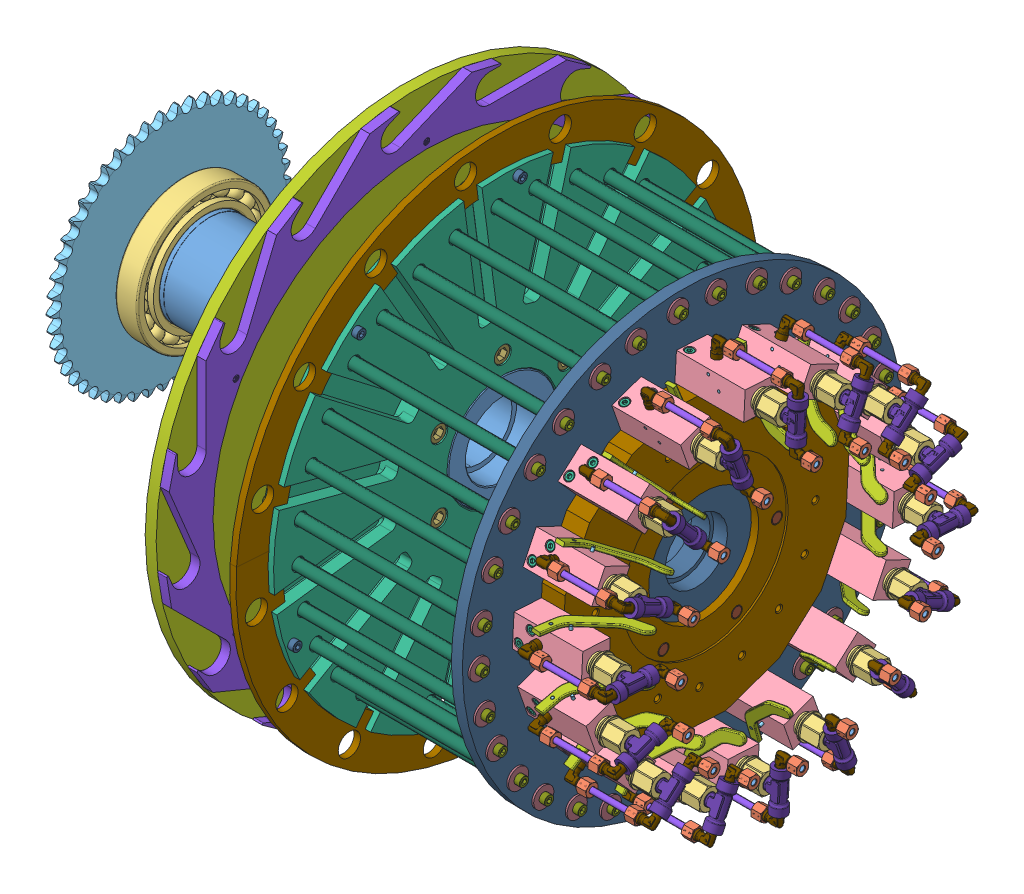
SolidWorks assembly assieme parte rotante, configuration Default. Lengths in mm. (continued)
Components (placement in the parent): (continued)
- AssiemeValvola-7: AssiemeValvola [Default] at (515.3257 -134.8578 488.6421) x (0 0.901303 -0.433189) z (0 -0.433189 -0.901303) size (90.26 138.63 38)
  - RaccordoT-1: RaccordoT [Default] at origin size (43 29.75 16.5)
  - Raccordo a L-1: Raccordo a L [Default] at (-30 0 0) x (0 -1 0) z (0 0 -1) size (28.34 25.51 14.01)
    - 1809_06_10_01-1: 1809_06_10_01 [Default] at origin size (22.49 23 10)
    - 1809_06_10_02-1: 1809_06_10_02 [Default] at origin size (6.5 8.5 8.5)
    - 1809_06_10_03-1: 1809_06_10_03 [Default] at origin size (11.02 15.01 14.01)
  - Raccordo a L-2: Raccordo a L [Default] at (30 0 0) x (0 1 0) z (0 0 -1) size (28.34 25.51 14.01)
    - 1809_06_10_01-1: 1809_06_10_01 [Default] at origin size (22.49 23 10)
    - 1809_06_10_02-1: 1809_06_10_02 [Default] at origin size (6.5 8.5 8.5)
    - 1809_06_10_03-1: 1809_06_10_03 [Default] at origin size (11.02 15.01 14.01)
  - TappoChiusura-1: TappoChiusura [Default] at (0 -32 0) x (0 -1 0) z (0 0 1) size (38.28 26.74 26.74)
  - CorpoValvola-1: CorpoValvola [Default] at (-15 -115.2824 0) size (30 75 34)
  - Raccordo a L-3: Raccordo a L [Default] at (-30 -88.2824 0) x (0 1 0) z (0 0 1) size (28.34 25.51 14.01)
    - 1809_06_10_01-1: 1809_06_10_01 [Default] at origin size (22.49 23 10)
    - 1809_06_10_02-1: 1809_06_10_02 [Default] at origin size (6.5 8.5 8.5)
    - 1809_06_10_03-1: 1809_06_10_03 [Default] at origin size (11.02 15.01 14.01)
  - Spina_3x38-1: Spina_3x38 [Default] at (0 -68.2824 -21) x (-1 0 0) z (0 0 1) size (3 3 38)
  - Spina_3x38-2: Spina_3x38 [Default] at (-10 -80.2824 -21) x (0.996193 0.087174 0) z (0 0 1) size (3 3 38)
  - M5 40mm-3: M5 40mm [ISO 4762 M5 x 40 - 40N] at (-14.6 -108.7824 9) size (45 8.5 8.5)
  - M5 40mm-2: M5 40mm [ISO 4762 M5 x 40 - 40N] at (-14.6 -96.7824 -9) size (45 8.5 8.5)
  - LevaValvola-1: LevaValvola [Default] at (-24.507 -86.571 -17) x (0.996193 0.087174 0) z (0 0 1) size (77.55 60.2 4)
  - Tubo-1: Tubo [Default] at (-30 -15.9665 0) x (1 0 0) z (0 -1 0) size (6 6 56.4)
- AssiemeValvola-8: AssiemeValvola [Default] at (515.3257 -95.0129 541.6718) x (0 0.666921 -0.745128) z (0 -0.745128 -0.666921) size (90.26 138.63 38)
  - RaccordoT-1: RaccordoT [Default] at origin size (43 29.75 16.5)
  - Raccordo a L-1: Raccordo a L [Default] at (-30 0 0) x (0 -1 0) z (0 0 -1) size (28.34 25.51 14.01)
    - 1809_06_10_01-1: 1809_06_10_01 [Default] at origin size (22.49 23 10)
    - 1809_06_10_02-1: 1809_06_10_02 [Default] at origin size (6.5 8.5 8.5)
    - 1809_06_10_03-1: 1809_06_10_03 [Default] at origin size (11.02 15.01 14.01)
  - Raccordo a L-2: Raccordo a L [Default] at (30 0 0) x (0 1 0) z (0 0 -1) size (28.34 25.51 14.01)
    - 1809_06_10_01-1: 1809_06_10_01 [Default] at origin size (22.49 23 10)
    - 1809_06_10_02-1: 1809_06_10_02 [Default] at origin size (6.5 8.5 8.5)
    - 1809_06_10_03-1: 1809_06_10_03 [Default] at origin size (11.02 15.01 14.01)
  - TappoChiusura-1: TappoChiusura [Default] at (0 -32 0) x (0 -1 0) z (0 0 1) size (38.28 26.74 26.74)
  - CorpoValvola-1: CorpoValvola [Default] at (-15 -115.2824 0) size (30 75 34)
  - Raccordo a L-3: Raccordo a L [Default] at (-30 -88.2824 0) x (0 1 0) z (0 0 1) size (28.34 25.51 14.01)
    - 1809_06_10_01-1: 1809_06_10_01 [Default] at origin size (22.49 23 10)
    - 1809_06_10_02-1: 1809_06_10_02 [Default] at origin size (6.5 8.5 8.5)
    - 1809_06_10_03-1: 1809_06_10_03 [Default] at origin size (11.02 15.01 14.01)
  - Spina_3x38-1: Spina_3x38 [Default] at (0 -68.2824 -21) x (-1 0 0) z (0 0 1) size (3 3 38)
  - Spina_3x38-2: Spina_3x38 [Default] at (-10 -80.2824 -21) x (0.996193 0.087174 0) z (0 0 1) size (3 3 38)
  - M5 40mm-3: M5 40mm [ISO 4762 M5 x 40 - 40N] at (-14.6 -108.7824 9) size (45 8.5 8.5)
  - M5 40mm-2: M5 40mm [ISO 4762 M5 x 40 - 40N] at (-14.6 -96.7824 -9) size (45 8.5 8.5)
  - LevaValvola-1: LevaValvola [Default] at (-24.507 -86.571 -17) x (0.996193 0.087174 0) z (0 0 1) size (77.55 60.2 4)
  - Tubo-1: Tubo [Default] at (-30 -15.9665 0) x (1 0 0) z (0 -1 0) size (6 6 56.4)
- AssiemeValvola-9: AssiemeValvola [Default] at (515.3257 -37.9074 575.4168) x (0 0.331007 -0.943628) z (0 -0.943628 -0.331007) size (90.26 138.63 38)
  - RaccordoT-1: RaccordoT [Default] at origin size (43 29.75 16.5)
  - Raccordo a L-1: Raccordo a L [Default] at (-30 0 0) x (0 -1 0) z (0 0 -1) size (28.34 25.51 14.01)
    - 1809_06_10_01-1: 1809_06_10_01 [Default] at origin size (22.49 23 10)
    - 1809_06_10_02-1: 1809_06_10_02 [Default] at origin size (6.5 8.5 8.5)
    - 1809_06_10_03-1: 1809_06_10_03 [Default] at origin size (11.02 15.01 14.01)
  - Raccordo a L-2: Raccordo a L [Default] at (30 0 0) x (0 1 0) z (0 0 -1) size (28.34 25.51 14.01)
    - 1809_06_10_01-1: 1809_06_10_01 [Default] at origin size (22.49 23 10)
    - 1809_06_10_02-1: 1809_06_10_02 [Default] at origin size (6.5 8.5 8.5)
    - 1809_06_10_03-1: 1809_06_10_03 [Default] at origin size (11.02 15.01 14.01)
  - TappoChiusura-1: TappoChiusura [Default] at (0 -32 0) x (0 -1 0) z (0 0 1) size (38.28 26.74 26.74)
  - CorpoValvola-1: CorpoValvola [Default] at (-15 -115.2824 0) size (30 75 34)
  - Raccordo a L-3: Raccordo a L [Default] at (-30 -88.2824 0) x (0 1 0) z (0 0 1) size (28.34 25.51 14.01)
    - 1809_06_10_01-1: 1809_06_10_01 [Default] at origin size (22.49 23 10)
    - 1809_06_10_02-1: 1809_06_10_02 [Default] at origin size (6.5 8.5 8.5)
    - 1809_06_10_03-1: 1809_06_10_03 [Default] at origin size (11.02 15.01 14.01)
  - Spina_3x38-1: Spina_3x38 [Default] at (0 -68.2824 -21) x (-1 0 0) z (0 0 1) size (3 3 38)
  - Spina_3x38-2: Spina_3x38 [Default] at (-10 -80.2824 -21) x (0.996193 0.087174 0) z (0 0 1) size (3 3 38)
  - M5 40mm-3: M5 40mm [ISO 4762 M5 x 40 - 40N] at (-14.6 -108.7824 9) size (45 8.5 8.5)
  - M5 40mm-2: M5 40mm [ISO 4762 M5 x 40 - 40N] at (-14.6 -96.7824 -9) size (45 8.5 8.5)
  - LevaValvola-1: LevaValvola [Default] at (-24.507 -86.571 -17) x (0.996193 0.087174 0) z (0 0 1) size (77.55 60.2 4)
  - Tubo-1: Tubo [Default] at (-30 -15.9665 0) x (1 0 0) z (0 -1 0) size (6 6 56.4)
- AssiemeValvola-10: AssiemeValvola [Default] at (515.3257 27.7648 584.7399) x (0 -0.055301 -0.99847) z (0 -0.99847 0.055301) size (90.26 138.63 38)
  - RaccordoT-1: RaccordoT [Default] at origin size (43 29.75 16.5)
  - Raccordo a L-1: Raccordo a L [Default] at (-30 0 0) x (0 -1 0) z (0 0 -1) size (28.34 25.51 14.01)
    - 1809_06_10_01-1: 1809_06_10_01 [Default] at origin size (22.49 23 10)
    - 1809_06_10_02-1: 1809_06_10_02 [Default] at origin size (6.5 8.5 8.5)
    - 1809_06_10_03-1: 1809_06_10_03 [Default] at origin size (11.02 15.01 14.01)
  - Raccordo a L-2: Raccordo a L [Default] at (30 0 0) x (0 1 0) z (0 0 -1) size (28.34 25.51 14.01)
    - 1809_06_10_01-1: 1809_06_10_01 [Default] at origin size (22.49 23 10)
    - 1809_06_10_02-1: 1809_06_10_02 [Default] at origin size (6.5 8.5 8.5)
    - 1809_06_10_03-1: 1809_06_10_03 [Default] at origin size (11.02 15.01 14.01)
  - TappoChiusura-1: TappoChiusura [Default] at (0 -32 0) x (0 -1 0) z (0 0 1) size (38.28 26.74 26.74)
  - CorpoValvola-1: CorpoValvola [Default] at (-15 -115.2824 0) size (30 75 34)
  - Raccordo a L-3: Raccordo a L [Default] at (-30 -88.2824 0) x (0 1 0) z (0 0 1) size (28.34 25.51 14.01)
    - 1809_06_10_01-1: 1809_06_10_01 [Default] at origin size (22.49 23 10)
    - 1809_06_10_02-1: 1809_06_10_02 [Default] at origin size (6.5 8.5 8.5)
    - 1809_06_10_03-1: 1809_06_10_03 [Default] at origin size (11.02 15.01 14.01)
  - Spina_3x38-1: Spina_3x38 [Default] at (0 -68.2824 -21) x (-1 0 0) z (0 0 1) size (3 3 38)
  - Spina_3x38-2: Spina_3x38 [Default] at (-10 -80.2824 -21) x (0.996193 0.087174 0) z (0 0 1) size (3 3 38)
  - M5 40mm-3: M5 40mm [ISO 4762 M5 x 40 - 40N] at (-14.6 -108.7824 9) size (45 8.5 8.5)
  - M5 40mm-2: M5 40mm [ISO 4762 M5 x 40 - 40N] at (-14.6 -96.7824 -9) size (45 8.5 8.5)
  - LevaValvola-1: LevaValvola [Default] at (-24.507 -86.571 -17) x (0.996193 0.087174 0) z (0 0 1) size (77.55 60.2 4)
  - Tubo-1: Tubo [Default] at (-30 -15.9665 0) x (1 0 0) z (0 -1 0) size (6 6 56.4)
- AssiemeValvola-11: AssiemeValvola [Default] at (515.3257 92.0058 568.2215) x (0 -0.433189 -0.901303) z (0 -0.901303 0.433189) size (90.26 138.63 38)
  - RaccordoT-1: RaccordoT [Default] at origin size (43 29.75 16.5)
  - Raccordo a L-1: Raccordo a L [Default] at (-30 0 0) x (0 -1 0) z (0 0 -1) size (28.34 25.51 14.01)
    - 1809_06_10_01-1: 1809_06_10_01 [Default] at origin size (22.49 23 10)
    - 1809_06_10_02-1: 1809_06_10_02 [Default] at origin size (6.5 8.5 8.5)
    - 1809_06_10_03-1: 1809_06_10_03 [Default] at origin size (11.02 15.01 14.01)
  - Raccordo a L-2: Raccordo a L [Default] at (30 0 0) x (0 1 0) z (0 0 -1) size (28.34 25.51 14.01)
    - 1809_06_10_01-1: 1809_06_10_01 [Default] at origin size (22.49 23 10)
    - 1809_06_10_02-1: 1809_06_10_02 [Default] at origin size (6.5 8.5 8.5)
    - 1809_06_10_03-1: 1809_06_10_03 [Default] at origin size (11.02 15.01 14.01)
  - TappoChiusura-1: TappoChiusura [Default] at (0 -32 0) x (0 -1 0) z (0 0 1) size (38.28 26.74 26.74)
  - CorpoValvola-1: CorpoValvola [Default] at (-15 -115.2824 0) size (30 75 34)
  - Raccordo a L-3: Raccordo a L [Default] at (-30 -88.2824 0) x (0 1 0) z (0 0 1) size (28.34 25.51 14.01)
    - 1809_06_10_01-1: 1809_06_10_01 [Default] at origin size (22.49 23 10)
    - 1809_06_10_02-1: 1809_06_10_02 [Default] at origin size (6.5 8.5 8.5)
    - 1809_06_10_03-1: 1809_06_10_03 [Default] at origin size (11.02 15.01 14.01)
  - Spina_3x38-1: Spina_3x38 [Default] at (0 -68.2824 -21) x (-1 0 0) z (0 0 1) size (3 3 38)
  - Spina_3x38-2: Spina_3x38 [Default] at (-10 -80.2824 -21) x (0.996193 0.087174 0) z (0 0 1) size (3 3 38)
  - M5 40mm-3: M5 40mm [ISO 4762 M5 x 40 - 40N] at (-14.6 -108.7824 9) size (45 8.5 8.5)
  - M5 40mm-2: M5 40mm [ISO 4762 M5 x 40 - 40N] at (-14.6 -96.7824 -9) size (45 8.5 8.5)
  - LevaValvola-1: LevaValvola [Default] at (-24.507 -86.571 -17) x (0.996193 0.087174 0) z (0 0 1) size (77.55 60.2 4)
  - Tubo-1: Tubo [Default] at (-30 -15.9665 0) x (1 0 0) z (0 -1 0) size (6 6 56.4)
- AssiemeValvola-12: AssiemeValvola [Default] at (515.3257 145.0355 528.3766) x (0 -0.745128 -0.666921) z (0 -0.666921 0.745128) size (90.26 138.63 38)
  - RaccordoT-1: RaccordoT [Default] at origin size (43 29.75 16.5)
  - Raccordo a L-1: Raccordo a L [Default] at (-30 0 0) x (0 -1 0) z (0 0 -1) size (28.34 25.51 14.01)
    - 1809_06_10_01-1: 1809_06_10_01 [Default] at origin size (22.49 23 10)
    - 1809_06_10_02-1: 1809_06_10_02 [Default] at origin size (6.5 8.5 8.5)
    - 1809_06_10_03-1: 1809_06_10_03 [Default] at origin size (11.02 15.01 14.01)
  - Raccordo a L-2: Raccordo a L [Default] at (30 0 0) x (0 1 0) z (0 0 -1) size (28.34 25.51 14.01)
    - 1809_06_10_01-1: 1809_06_10_01 [Default] at origin size (22.49 23 10)
    - 1809_06_10_02-1: 1809_06_10_02 [Default] at origin size (6.5 8.5 8.5)
    - 1809_06_10_03-1: 1809_06_10_03 [Default] at origin size (11.02 15.01 14.01)
  - TappoChiusura-1: TappoChiusura [Default] at (0 -32 0) x (0 -1 0) z (0 0 1) size (38.28 26.74 26.74)
  - CorpoValvola-1: CorpoValvola [Default] at (-15 -115.2824 0) size (30 75 34)
  - Raccordo a L-3: Raccordo a L [Default] at (-30 -88.2824 0) x (0 1 0) z (0 0 1) size (28.34 25.51 14.01)
    - 1809_06_10_01-1: 1809_06_10_01 [Default] at origin size (22.49 23 10)
    - 1809_06_10_02-1: 1809_06_10_02 [Default] at origin size (6.5 8.5 8.5)
    - 1809_06_10_03-1: 1809_06_10_03 [Default] at origin size (11.02 15.01 14.01)
  - Spina_3x38-1: Spina_3x38 [Default] at (0 -68.2824 -21) x (-1 0 0) z (0 0 1) size (3 3 38)
  - Spina_3x38-2: Spina_3x38 [Default] at (-10 -80.2824 -21) x (0.996193 0.087174 0) z (0 0 1) size (3 3 38)
  - M5 40mm-3: M5 40mm [ISO 4762 M5 x 40 - 40N] at (-14.6 -108.7824 9) size (45 8.5 8.5)
  - M5 40mm-2: M5 40mm [ISO 4762 M5 x 40 - 40N] at (-14.6 -96.7824 -9) size (45 8.5 8.5)
  - LevaValvola-1: LevaValvola [Default] at (-24.507 -86.571 -17) x (0.996193 0.087174 0) z (0 0 1) size (77.55 60.2 4)
  - Tubo-1: Tubo [Default] at (-30 -15.9665 0) x (1 0 0) z (0 -1 0) size (6 6 56.4)
- AssiemeValvola-13: AssiemeValvola [Default] at (515.3257 178.7805 471.2711) x (0 -0.943628 -0.331007) z (0 -0.331007 0.943628) size (90.26 138.63 38)
  - RaccordoT-1: RaccordoT [Default] at origin size (43 29.75 16.5)
  - Raccordo a L-1: Raccordo a L [Default] at (-30 0 0) x (0 -1 0) z (0 0 -1) size (28.34 25.51 14.01)
    - 1809_06_10_01-1: 1809_06_10_01 [Default] at origin size (22.49 23 10)
    - 1809_06_10_02-1: 1809_06_10_02 [Default] at origin size (6.5 8.5 8.5)
    - 1809_06_10_03-1: 1809_06_10_03 [Default] at origin size (11.02 15.01 14.01)
  - Raccordo a L-2: Raccordo a L [Default] at (30 0 0) x (0 1 0) z (0 0 -1) size (28.34 25.51 14.01)
    - 1809_06_10_01-1: 1809_06_10_01 [Default] at origin size (22.49 23 10)
    - 1809_06_10_02-1: 1809_06_10_02 [Default] at origin size (6.5 8.5 8.5)
    - 1809_06_10_03-1: 1809_06_10_03 [Default] at origin size (11.02 15.01 14.01)
  - TappoChiusura-1: TappoChiusura [Default] at (0 -32 0) x (0 -1 0) z (0 0 1) size (38.28 26.74 26.74)
  - CorpoValvola-1: CorpoValvola [Default] at (-15 -115.2824 0) size (30 75 34)
  - Raccordo a L-3: Raccordo a L [Default] at (-30 -88.2824 0) x (0 1 0) z (0 0 1) size (28.34 25.51 14.01)
    - 1809_06_10_01-1: 1809_06_10_01 [Default] at origin size (22.49 23 10)
    - 1809_06_10_02-1: 1809_06_10_02 [Default] at origin size (6.5 8.5 8.5)
    - 1809_06_10_03-1: 1809_06_10_03 [Default] at origin size (11.02 15.01 14.01)
  - Spina_3x38-1: Spina_3x38 [Default] at (0 -68.2824 -21) x (-1 0 0) z (0 0 1) size (3 3 38)
  - Spina_3x38-2: Spina_3x38 [Default] at (-10 -80.2824 -21) x (0.996193 0.087174 0) z (0 0 1) size (3 3 38)
  - M5 40mm-3: M5 40mm [ISO 4762 M5 x 40 - 40N] at (-14.6 -108.7824 9) size (45 8.5 8.5)
  - M5 40mm-2: M5 40mm [ISO 4762 M5 x 40 - 40N] at (-14.6 -96.7824 -9) size (45 8.5 8.5)
  - LevaValvola-1: LevaValvola [Default] at (-24.507 -86.571 -17) x (0.996193 0.087174 0) z (0 0 1) size (77.55 60.2 4)
  - Tubo-1: Tubo [Default] at (-30 -15.9665 0) x (1 0 0) z (0 -1 0) size (6 6 56.4)
- AssiemeValvola-14: AssiemeValvola [Default] at (515.3257 188.1036 405.5989) x (0 -0.99847 0.055301) z (0 0.055301 0.99847) size (90.26 138.63 38)
  - RaccordoT-1: RaccordoT [Default] at origin size (43 29.75 16.5)
  - Raccordo a L-1: Raccordo a L [Default] at (-30 0 0) x (0 -1 0) z (0 0 -1) size (28.34 25.51 14.01)
    - 1809_06_10_01-1: 1809_06_10_01 [Default] at origin size (22.49 23 10)
    - 1809_06_10_02-1: 1809_06_10_02 [Default] at origin size (6.5 8.5 8.5)
    - 1809_06_10_03-1: 1809_06_10_03 [Default] at origin size (11.02 15.01 14.01)
  - Raccordo a L-2: Raccordo a L [Default] at (30 0 0) x (0 1 0) z (0 0 -1) size (28.34 25.51 14.01)
    - 1809_06_10_01-1: 1809_06_10_01 [Default] at origin size (22.49 23 10)
    - 1809_06_10_02-1: 1809_06_10_02 [Default] at origin size (6.5 8.5 8.5)
    - 1809_06_10_03-1: 1809_06_10_03 [Default] at origin size (11.02 15.01 14.01)
  - TappoChiusura-1: TappoChiusura [Default] at (0 -32 0) x (0 -1 0) z (0 0 1) size (38.28 26.74 26.74)
  - CorpoValvola-1: CorpoValvola [Default] at (-15 -115.2824 0) size (30 75 34)
  - Raccordo a L-3: Raccordo a L [Default] at (-30 -88.2824 0) x (0 1 0) z (0 0 1) size (28.34 25.51 14.01)
    - 1809_06_10_01-1: 1809_06_10_01 [Default] at origin size (22.49 23 10)
    - 1809_06_10_02-1: 1809_06_10_02 [Default] at origin size (6.5 8.5 8.5)
    - 1809_06_10_03-1: 1809_06_10_03 [Default] at origin size (11.02 15.01 14.01)
  - Spina_3x38-1: Spina_3x38 [Default] at (0 -68.2824 -21) x (-1 0 0) z (0 0 1) size (3 3 38)
  - Spina_3x38-2: Spina_3x38 [Default] at (-10 -80.2824 -21) x (0.996193 0.087174 0) z (0 0 1) size (3 3 38)
  - M5 40mm-3: M5 40mm [ISO 4762 M5 x 40 - 40N] at (-14.6 -108.7824 9) size (45 8.5 8.5)
  - M5 40mm-2: M5 40mm [ISO 4762 M5 x 40 - 40N] at (-14.6 -96.7824 -9) size (45 8.5 8.5)
  - LevaValvola-1: LevaValvola [Default] at (-24.507 -86.571 -17) x (0.996193 0.087174 0) z (0 0 1) size (77.55 60.2 4)
  - Tubo-1: Tubo [Default] at (-30 -15.9665 0) x (1 0 0) z (0 -1 0) size (6 6 56.4)
- AssiemeValvola-15: AssiemeValvola [Default] at (515.3257 171.5852 341.3579) x (0 -0.901303 0.433189) z (0 0.433189 0.901303) size (90.26 138.63 38)
  - RaccordoT-1: RaccordoT [Default] at origin size (43 29.75 16.5)
  - Raccordo a L-1: Raccordo a L [Default] at (-30 0 0) x (0 -1 0) z (0 0 -1) size (28.34 25.51 14.01)
    - 1809_06_10_01-1: 1809_06_10_01 [Default] at origin size (22.49 23 10)
    - 1809_06_10_02-1: 1809_06_10_02 [Default] at origin size (6.5 8.5 8.5)
    - 1809_06_10_03-1: 1809_06_10_03 [Default] at origin size (11.02 15.01 14.01)
  - Raccordo a L-2: Raccordo a L [Default] at (30 0 0) x (0 1 0) z (0 0 -1) size (28.34 25.51 14.01)
    - 1809_06_10_01-1: 1809_06_10_01 [Default] at origin size (22.49 23 10)
    - 1809_06_10_02-1: 1809_06_10_02 [Default] at origin size (6.5 8.5 8.5)
    - 1809_06_10_03-1: 1809_06_10_03 [Default] at origin size (11.02 15.01 14.01)
  - TappoChiusura-1: TappoChiusura [Default] at (0 -32 0) x (0 -1 0) z (0 0 1) size (38.28 26.74 26.74)
  - CorpoValvola-1: CorpoValvola [Default] at (-15 -115.2824 0) size (30 75 34)
  - Raccordo a L-3: Raccordo a L [Default] at (-30 -88.2824 0) x (0 1 0) z (0 0 1) size (28.34 25.51 14.01)
    - 1809_06_10_01-1: 1809_06_10_01 [Default] at origin size (22.49 23 10)
    - 1809_06_10_02-1: 1809_06_10_02 [Default] at origin size (6.5 8.5 8.5)
    - 1809_06_10_03-1: 1809_06_10_03 [Default] at origin size (11.02 15.01 14.01)
  - Spina_3x38-1: Spina_3x38 [Default] at (0 -68.2824 -21) x (-1 0 0) z (0 0 1) size (3 3 38)
  - Spina_3x38-2: Spina_3x38 [Default] at (-10 -80.2824 -21) x (0.996193 0.087174 0) z (0 0 1) size (3 3 38)
  - M5 40mm-3: M5 40mm [ISO 4762 M5 x 40 - 40N] at (-14.6 -108.7824 9) size (45 8.5 8.5)
  - M5 40mm-2: M5 40mm [ISO 4762 M5 x 40 - 40N] at (-14.6 -96.7824 -9) size (45 8.5 8.5)
  - LevaValvola-1: LevaValvola [Default] at (-24.507 -86.571 -17) x (0.996193 0.087174 0) z (0 0 1) size (77.55 60.2 4)
  - Tubo-1: Tubo [Default] at (-30 -15.9665 0) x (1 0 0) z (0 -1 0) size (6 6 56.4)
- AssiemeValvola-16: AssiemeValvola [Default] at (515.3257 131.7403 288.3282) x (0 -0.666921 0.745128) z (0 0.745128 0.666921) size (90.26 138.63 38)
  - RaccordoT-1: RaccordoT [Default] at origin size (43 29.75 16.5)
  - Raccordo a L-1: Raccordo a L [Default] at (-30 0 0) x (0 -1 0) z (0 0 -1) size (28.34 25.51 14.01)
    - 1809_06_10_01-1: 1809_06_10_01 [Default] at origin size (22.49 23 10)
    - 1809_06_10_02-1: 1809_06_10_02 [Default] at origin size (6.5 8.5 8.5)
    - 1809_06_10_03-1: 1809_06_10_03 [Default] at origin size (11.02 15.01 14.01)
  - Raccordo a L-2: Raccordo a L [Default] at (30 0 0) x (0 1 0) z (0 0 -1) size (28.34 25.51 14.01)
    - 1809_06_10_01-1: 1809_06_10_01 [Default] at origin size (22.49 23 10)
    - 1809_06_10_02-1: 1809_06_10_02 [Default] at origin size (6.5 8.5 8.5)
    - 1809_06_10_03-1: 1809_06_10_03 [Default] at origin size (11.02 15.01 14.01)
  - TappoChiusura-1: TappoChiusura [Default] at (0 -32 0) x (0 -1 0) z (0 0 1) size (38.28 26.74 26.74)
  - CorpoValvola-1: CorpoValvola [Default] at (-15 -115.2824 0) size (30 75 34)
  - Raccordo a L-3: Raccordo a L [Default] at (-30 -88.2824 0) x (0 1 0) z (0 0 1) size (28.34 25.51 14.01)
    - 1809_06_10_01-1: 1809_06_10_01 [Default] at origin size (22.49 23 10)
    - 1809_06_10_02-1: 1809_06_10_02 [Default] at origin size (6.5 8.5 8.5)
    - 1809_06_10_03-1: 1809_06_10_03 [Default] at origin size (11.02 15.01 14.01)
  - Spina_3x38-1: Spina_3x38 [Default] at (0 -68.2824 -21) x (-1 0 0) z (0 0 1) size (3 3 38)
  - Spina_3x38-2: Spina_3x38 [Default] at (-10 -80.2824 -21) x (0.996193 0.087174 0) z (0 0 1) size (3 3 38)
  - M5 40mm-3: M5 40mm [ISO 4762 M5 x 40 - 40N] at (-14.6 -108.7824 9) size (45 8.5 8.5)
  - M5 40mm-2: M5 40mm [ISO 4762 M5 x 40 - 40N] at (-14.6 -96.7824 -9) size (45 8.5 8.5)
  - LevaValvola-1: LevaValvola [Default] at (-24.507 -86.571 -17) x (0.996193 0.087174 0) z (0 0 1) size (77.55 60.2 4)
  - Tubo-1: Tubo [Default] at (-30 -15.9665 0) x (1 0 0) z (0 -1 0) size (6 6 56.4)
- Disco alimentazione guarnizione fi24.4-1: Disco alimentazione guarnizione fi24.4 [Default] at (198.0433 18.3637 415) x (0 0.065403 0.997859) z (-1 0 0) size (570 285 7.35)
- Disco alimentazione guarnizione fi24.4-2: Disco alimentazione guarnizione fi24.4 [Default] at (198.0433 18.3637 415) x (0 -0.065403 -0.997859) z (-1 0 0) size (570 285 7.35)
- m6 12mm-1: m6 12mm [ISO 4762 M6 x 12 - 12N] at (210.0433 200.6849 574.8914) x (-1 0 0) z (0 0.793353 -0.608761) size (18 10 10)
- m6 12mm-7: m6 12mm [ISO 4762 M6 x 12 - 12N] at (210.0433 260.3445 399.1397) x (-1 0 0) z (0 0.793353 -0.608761) size (18 10 10)
- m6 12mm-8: m6 12mm [ISO 4762 M6 x 12 - 12N] at (210.0433 96.3128 185.3694) x (-1 0 0) z (0 0.793353 -0.608761) size (18 10 10)
- m6 12mm-9: m6 12mm [ISO 4762 M6 x 12 - 12N] at (210.0433 -59.5854 644.6306) x (-1 0 0) z (0 -0.793353 -0.608761) size (18 10 10)
- m6 12mm-10: m6 12mm [ISO 4762 M6 x 12 - 12N] at (210.0433 -223.6171 430.8603) x (-1 0 0) z (0 -0.793353 -0.608761) size (18 10 10)
- m6 12mm-11: m6 12mm [ISO 4762 M6 x 12 - 12N] at (210.0433 -163.9575 255.1086) x (-1 0 0) z (0 0.793353 -0.608761) size (18 10 10)
Mates (geometry in assembly coordinates):
- Concentrico1: concentric anti-aligned: circle of albero rotazione piatti-1; circle of seger 100mm-1
- Coincidente1: coincident anti-aligned: plane of albero rotazione piatti-1 through (-143.4567 18.3637 415) normal (-1 0 0); plane of c-type retaining ring_external_ks-1 through (-143.4567 18.3637 415) normal (1 0 0)
- Coincidente2: coincident aligned: plane of albero rotazione piatti-1 through (60.413 18.3637 415) normal (0 1 0); plane of c-type retaining ring_external_ks-1 through (-146.4567 18.3637 415) normal (0 1 0)
- Concentrico21: concentric aligned: cylinder of albero rotazione piatti-1 through (60.413 18.3637 415) axis (1 0 0) radius 50; cylinder of SKF - 6020 - 20,DE,NC,20_68-1 through (-152.0942 18.3637 415) axis (1 0 0) radius 50
- Coincidente3: coincident anti-aligned: plane of c-type retaining ring_external_ks-1 through (-143.4567 18.3637 415) normal (1 0 0); plane of SKF - 6020 - 20,DE,NC,20_68-1 through (-143.4567 -33.4256 439.9823) normal (-1 0 0)
- Concentrico3: concentric aligned: cylinder of albero rotazione piatti-1 through (60.413 18.3637 415) axis (1 0 0) radius 47.5; cylinder of calettatore d95-1 through (-188.8867 18.3637 415) axis (1 0 0) radius 47.5
- Coincidente7: coincident aligned: plane of albero rotazione piatti-1 through (60.413 18.3637 415) normal (0 1 0); plane of calettatore d95-1 through (-173.8867 18.3637 415) normal (0 1 0)
- Concentrico5: concentric aligned: cylinder of albero rotazione piatti-1 through (60.413 18.3637 415) axis (1 0 0) radius 49.75; cylinder of SKF - 6020 - 20,DE,NC,20_68-2 through (41.4058 18.3637 415) axis (1 0 0) radius 50
- Coincidente8: coincident anti-aligned: plane of albero rotazione piatti-1 through (74.0433 18.3637 415) normal (-1 0 0); plane of SKF - 6020 - 20,DE,NC,20_68-2 through (74.0433 -28.0673 437.2803) normal (1 0 0)
- Concentrico6: concentric aligned: cylinder of albero rotazione piatti-1 through (60.413 18.3637 415) axis (1 0 0) radius 60; cylinder of Disco supporto montaggio e Colonne-1 through (5.3377 18.3637 415) axis (1 0 0) radius 60
- Concentrico7: concentric aligned: cylinder of albero rotazione piatti-1 through (101.3656 98.3637 415) axis (1 0 0) radius 6.25; cylinder of Disco supporto montaggio e Colonne-1 through (204.0433 98.3637 415) axis (1 0 0) radius 9.25
- Coincidente9: coincident anti-aligned: plane of albero rotazione piatti-1 through (175.0433 18.3637 415) normal (1 0 0); plane of Disco supporto montaggio e Colonne-1 through (175.0433 18.3637 415) normal (-1 0 0)
- Concentrico8: concentric anti-aligned: cylinder of albero rotazione piatti-1 through (60.413 18.3637 415) axis (1 0 0) radius 60; cylinder of piatto rotante porta tappi-1 through (111.0433 18.3637 415) axis (-1 0 0) radius 60
- Concentrico9: concentric aligned: circle of albero rotazione piatti-1; circle of piatto rotante porta tappi-1
- Coincidente10: coincident anti-aligned: plane of albero rotazione piatti-1 through (119.0433 18.3637 415) normal (-1 0 0); plane of piatto rotante porta tappi-1 through (119.0433 18.3637 415) normal (1 0 0)
- Concentrico10: concentric aligned: cylinder of piatto rotante porta tappi-1 through (119.0433 18.3637 415) axis (-1 0 0) radius 233; cylinder of disco trasportatore tappi 31-1 through (121.0433 18.3637 415) axis (-1 0 0) radius 233
- Tangente2: tangent: cylinder of piatto rotante porta tappi-1 through (98.5243 -101.6363 622.8461) axis (1 0 0) radius 3.25; curve of disco trasportatore tappi 31-1
- Coincidente13: coincident anti-aligned: plane of piatto rotante porta tappi-1 through (111.0433 18.3637 415) normal (1 0 0); plane of disco trasportatore tappi 31-1 through (111.0433 18.3637 415) normal (-1 0 0)
- Concentrico11: concentric anti-aligned: cylinder of albero rotazione piatti-1 through (60.413 18.3637 415) axis (1 0 0) radius 40; cylinder of disco trascinato porta distributore vuoto-1 through (400.0433 18.3637 415) axis (-1 0 0) radius 30
- Concentrico12: concentric anti-aligned: cylinder of Disco supporto montaggio e Colonne-1 through (204.0433 -202.0247 450.2415) axis (1 0 0) radius 6; cylinder of disco trascinato porta distributore vuoto-1 through (417.0139 -202.0247 450.2415) axis (-1 0 0) radius 6
- Coincidente14: coincident anti-aligned: plane of Distributore Rotante-1 through (400.0433 18.3637 415) normal (-1 0 0); plane of disco trascinato porta distributore vuoto-1 through (400.0433 18.3637 415) normal (1 0 0)
- Concentrico13: concentric anti-aligned: circle of Distributore Rotante-1; circle of disco trascinato porta distributore vuoto-1
- Concentrico14: concentric anti-aligned: cylinder of Distributore Rotante-1 through (230.3377 18.3637 415) axis (1 0 0) radius 60; cylinder of disco trascinato porta distributore vuoto-1 through (415.0433 18.3637 415) axis (-1 0 0) radius 67.5
- Concentrico15: concentric anti-aligned: cylinder of disco trascinato porta distributore vuoto-1 through (388.0433 -53.0243 378.8925) axis (1 0 0) radius 6.25; cylinder of m12 35mm-1 through (344.2933 -53.0243 378.8925) axis (-1 0 0) radius 6
- Coincidente15: coincident anti-aligned: plane of disco trascinato porta distributore vuoto-1 through (388.0433 18.3637 415) normal (-1 0 0); plane of m12 35mm-1 through (388.0433 -45.2301 383.3925) normal (1 0 0)
- Parallelo1: parallel anti-aligned: plane of m12 35mm-1 through (382.0433 -47.9668 381.8125) normal (0 -1 0)
- Concentrico16: concentric aligned: cylinder of Disco supporto montaggio e Colonne-1 through (204.0433 -21.6363 345.718) axis (1 0 0) radius 9.25; cylinder of m12 90mm-3 through (234.7933 -21.6363 345.718) axis (1 0 0) radius 6
- Coincidente17: coincident anti-aligned: plane of Disco supporto montaggio e Colonne-1 through (191.0433 -27.049 342.593) normal (1 0 0); plane of m12 90mm-3 through (191.0433 -29.4305 341.218) normal (-1 0 0)
- Parallelo2: parallel aligned: plane of m12 35mm-1 through (382.0433 -47.9668 381.8125) normal (0 -1 0); plane of m12 90mm-3 through (197.0433 -16.5788 348.6379) normal (0 -1 0)
- Concentrico171: concentric anti-aligned: cylinder of piatto rotante porta tappi-1 through (98.5243 -101.6363 207.1539) axis (1 0 0) radius 3.25; cylinder of plain washer xlarge grade c_iso-1 through (64.1183 -101.6363 207.1539) axis (-1 0 0) radius 3.3
- Coincidente191: coincident anti-aligned: plane of piatto rotante porta tappi-1 through (99.0433 18.3637 415) normal (-1 0 0); plane of plain washer xlarge grade c_iso-1 through (99.0433 -101.6363 210.4539) normal (1 0 0)
- Parallelo3: parallel anti-aligned: plane of plain washer xlarge grade c_iso-1 through (99.0433 -101.6363 207.1539) normal (0 -1 0)
- Concentrico181: concentric aligned: cylinder of plain washer xlarge grade c_iso-1 through (64.1183 -101.6363 207.1539) axis (-1 0 0) radius 3.3; cylinder of M6 20mm-1 through (59.2933 -101.6363 207.1539) axis (-1 0 0) radius 5
- Coincidente211: coincident anti-aligned: plane of plain washer xlarge grade c_iso-1 through (97.0433 -101.6363 218.1539) normal (-1 0 0); plane of M6 20mm-1 through (97.0433 -97.3062 204.6539) normal (1 0 0)
- Parallelo4: parallel aligned: plane of m12 35mm-1 through (382.0433 -47.9668 381.8125) normal (0 -0.5 -0.866025); plane of M6 20mm-1 through (94.0433 -101.6363 210.0892) normal (0 -0.5 -0.866025)
- Concentrico19: concentric anti-aligned: cylinder of Disco supporto montaggio e Colonne-1 through (204.0433 70.1437 197.9013) axis (1 0 0) radius 6; cylinder of asta scorrimento carello-1 through (400.0433 70.1437 197.9013) axis (-1 0 0) radius 6
- Concentrico201: concentric aligned: cylinder of asta scorrimento carello-1 through (175.0433 70.1437 197.9013) axis (-1 0 0) radius 3.2; cylinder of plain washer xlarge grade c_iso-7 through (140.1183 70.1437 197.9013) axis (-1 0 0) radius 3.3
- Coincidente231: coincident anti-aligned: plane of asta scorrimento carello-1 through (175.0433 70.1437 197.9013) normal (-1 0 0); plane of plain washer xlarge grade c_iso-7 through (175.0433 70.1437 201.2013) normal (1 0 0)
- Concentrico211: concentric aligned: cylinder of plain washer xlarge grade c_iso-7 through (140.1183 70.1437 197.9013) axis (-1 0 0) radius 3.3; cylinder of M6 16mm-1 through (135.2933 70.1437 197.9013) axis (-1 0 0) radius 5
- Coincidente241: coincident anti-aligned: plane of plain washer xlarge grade c_iso-7 through (173.0433 70.1437 208.9013) normal (-1 0 0); plane of M6 16mm-1 through (173.0433 75.1437 197.9013) normal (1 0 0)
- Parallelo5: parallel aligned: plane of asta scorrimento carello-1 through (287.5433 70.1437 197.9013) normal (0 0 -1); plane of M6 16mm-1 through (170.0433 68.6761 200.4433) normal (0 0 -1)
- Parallelo9: parallel anti-aligned: plane of plain washer xlarge grade c_iso-7 through (175.0433 70.1437 197.9013) normal (0 0 1); plane of M6 16mm-1 through (170.0433 68.6761 200.4433) normal (0 0 -1)
- Coincidente30: coincident anti-aligned: plane of Disco supporto montaggio e Colonne-1 through (175.0433 18.3637 415) normal (-1 0 0); plane of plain washer xlarge grade c_iso-7 through (175.0433 70.1437 201.2013) normal (1 0 0)
- Coincidente31: coincident anti-aligned: plane of disco trascinato porta distributore vuoto-1 through (400.0433 18.3637 415) normal (1 0 0); plane of plain washer xlarge grade c_iso-26 through (400.0433 70.1437 201.2013) normal (-1 0 0)
- Coincidente32: coincident anti-aligned: plane of Distributore Rotante-1 through (400.0433 40.5763 258.5322) normal (0 0.331007 -0.943628); plane of AssiemeValvola-1/CorpoValvola-1 through (400.0433 85.7114 274.3647) normal (0 -0.331007 0.943628)
- Coincidente33: coincident anti-aligned: plane of disco trascinato porta distributore vuoto-1 through (400.0433 18.3637 415) normal (1 0 0); plane of AssiemeValvola-1/CorpoValvola-1 through (400.0433 95.6416 246.0559) normal (-1 0 0)
- Concentrico22: concentric anti-aligned: cylinder of Distributore Rotante-1 through (412.5433 55.4365 309.3136) axis (0 0.331007 -0.943628) radius 3; cylinder of AssiemeValvola-1/CorpoValvola-1 through (412.5433 69.6697 268.7376) axis (0 -0.331007 0.943628) radius 3
- Concentrico23: concentric anti-aligned: cylinder of Disco supporto montaggio e Colonne-1 through (198.0433 18.3637 415) axis (-1 0 0) radius 235; cylinder of Disco alimentazione guarnizione fi24.4-2 through (191.0433 18.3637 415) axis (1 0 0) radius 235
- Concentrico24: concentric anti-aligned: cylinder of Disco supporto montaggio e Colonne-1 through (198.0433 18.3637 415) axis (-1 0 0) radius 235; cylinder of Disco alimentazione guarnizione fi24.4-1 through (191.0433 18.3637 415) axis (1 0 0) radius 235
- Coincidente34: coincident anti-aligned: plane of Disco alimentazione guarnizione fi24.4-1 through (191.0433 33.7334 649.4968) normal (0 -0.997859 0.065403); plane of Disco alimentazione guarnizione fi24.4-2 through (191.0433 37.0036 699.3898) normal (0 0.997859 -0.065403)
- Coincidente35: coincident aligned: plane of Disco alimentazione guarnizione fi24.4-1 through (198.0433 18.3637 415) normal (1 0 0); plane of Disco alimentazione guarnizione fi24.4-2 through (198.0433 18.3637 415) normal (1 0 0)
- Concentrico25: concentric anti-aligned: cylinder of Disco supporto montaggio e Colonne-1 through (188.8509 -59.5854 644.6306) axis (1 0 0) radius 3.25; circle of Disco alimentazione guarnizione fi24.4-2
- Coincidente36: coincident anti-aligned: plane of Disco supporto montaggio e Colonne-1 through (198.0433 18.3637 415) normal (-1 0 0); plane of Disco alimentazione guarnizione fi24.4-2 through (198.0433 18.3637 415) normal (1 0 0)
- Concentrico26: concentric anti-aligned: cylinder of Disco supporto montaggio e Colonne-1 through (188.8509 200.6849 574.8914) axis (1 0 0) radius 3.25; cylinder of M6 16mm-65 through (198.0564 200.6849 574.8914) axis (-1 0 0) radius 3
- Concentrico271: concentric anti-aligned: cone of Disco supporto montaggio e Colonne-1 through (203.0433 200.6849 574.8914) axis (-1 0 0); cylinder of m6 12mm-1 through (241.7933 200.6849 574.8914) axis (1 0 0) radius 5
- Coincidente381: coincident anti-aligned: plane of Disco supporto montaggio e Colonne-1 through (204.0433 18.3637 415) normal (1 0 0); plane of m6 12mm-1 through (204.0433 203.7287 578.8581) normal (-1 0 0)
- Concentrico281: concentric anti-aligned: cone of Disco supporto montaggio e Colonne-1 through (203.0433 260.3445 399.1397) axis (-1 0 0); cylinder of m6 12mm-7 through (241.7933 260.3445 399.1397) axis (1 0 0) radius 5
- Coincidente401: coincident anti-aligned: plane of Disco supporto montaggio e Colonne-1 through (204.0433 18.3637 415) normal (1 0 0); plane of m6 12mm-7 through (204.0433 263.3883 403.1065) normal (-1 0 0)
- Parallelo11: parallel aligned: plane of m6 12mm-1 through (207.0433 198.898 572.5627) normal (0 0.92388 0.382683); plane of m6 12mm-7 through (207.0433 258.5576 396.8111) normal (0 0.92388 0.382683)
- Concentrico291: concentric anti-aligned: cone of Disco supporto montaggio e Colonne-1 through (203.0433 96.3128 185.3694) axis (-1 0 0); cylinder of m6 12mm-8 through (241.7933 96.3128 185.3694) axis (1 0 0) radius 5
- Coincidente421: coincident anti-aligned: plane of Disco supporto montaggio e Colonne-1 through (204.0433 18.3637 415) normal (1 0 0); plane of m6 12mm-8 through (204.0433 99.3566 189.3362) normal (-1 0 0)
- Coincidente44: coincident aligned: plane of m6 12mm-7 through (207.0433 259.2212 401.8516) normal (0 0.793353 -0.608761); plane of m6 12mm-8 through (207.0433 95.1895 188.0813) normal (0 0.793353 -0.608761)
- Concentrico301: concentric anti-aligned: cone of Disco supporto montaggio e Colonne-1 through (203.0433 -59.5854 644.6306) axis (-1 0 0); cylinder of m6 12mm-9 through (241.7933 -59.5854 644.6306) axis (1 0 0) radius 5
- Coincidente451: coincident anti-aligned: plane of Disco supporto montaggio e Colonne-1 through (204.0433 18.3637 415) normal (1 0 0); plane of m6 12mm-9 through (204.0433 -56.5416 640.6638) normal (-1 0 0)
- Concentrico311: concentric anti-aligned: cone of Disco supporto montaggio e Colonne-1 through (203.0433 -223.6171 430.8603) axis (-1 0 0); cylinder of m6 12mm-10 through (241.7933 -223.6171 430.8603) axis (1 0 0) radius 5
- Coincidente461: coincident anti-aligned: plane of Disco supporto montaggio e Colonne-1 through (204.0433 18.3637 415) normal (1 0 0); plane of m6 12mm-10 through (204.0433 -220.5733 426.8935) normal (-1 0 0)
- Concentrico321: concentric anti-aligned: cone of Disco supporto montaggio e Colonne-1 through (203.0433 -163.9575 255.1086) axis (-1 0 0); cylinder of m6 12mm-11 through (241.7933 -163.9575 255.1086) axis (1 0 0) radius 5
- Coincidente471: coincident anti-aligned: plane of Disco supporto montaggio e Colonne-1 through (204.0433 18.3637 415) normal (1 0 0); plane of m6 12mm-11 through (204.0433 -160.9136 259.0754) normal (-1 0 0)
- Parallelo13: parallel aligned: plane of m6 12mm-9 through (207.0433 -62.4955 644.2474) normal (0 0.92388 -0.382683); plane of m6 12mm-10 through (207.0433 -226.5272 430.4771) normal (0 0.92388 -0.382683)
- Parallelo14: parallel aligned: plane of Disco supporto montaggio e Colonne-1 through (191.0433 26.2972 408.9124) normal (0 -0.793353 0.608761); plane of m6 12mm-11 through (207.0433 -162.8342 252.3968) normal (0 -0.793353 0.608761)
- Parallelo15: parallel aligned: plane of Disco supporto montaggio e Colonne-1 through (191.0433 19.669 405.0856) normal (0 -0.130526 0.991445); plane of m6 12mm-10 through (207.0433 -221.8302 428.5316) normal (0 -0.130526 0.991445)
- Concentrico322: concentric anti-aligned: cylinder of albero rotazione piatti-1 through (60.413 18.3637 415) axis (1 0 0) radius 47.5; cylinder of Chain wheel ISO - 50Z 10A-1-1 through (-139.8862 18.3637 415) axis (-1 0 0) radius 47.5
- Coincidente472: coincident anti-aligned: plane of albero rotazione piatti-1 through (-155.9567 18.3637 415) normal (-1 0 0); plane of Chain wheel ISO - 50Z 10A-1-1 through (-155.9567 18.3637 415) normal (1 0 0)
- Parallelo16: parallel aligned: plane of Chain wheel ISO - 50Z 10A-1-1 through (-164.8867 18.3637 415) normal (0 1 0)
- Parallelo17: parallel aligned: plane of calettatore d95-1 through (-173.8867 18.3637 415) normal (0 1 0)
- Coincidente473: coincident anti-aligned: plane of calettatore d95-1 through (-159.8867 84.9137 415) normal (1 0 0); plane of Chain wheel ISO - 50Z 10A-1-1 through (-159.8867 18.3637 415) normal (-1 0 0)
